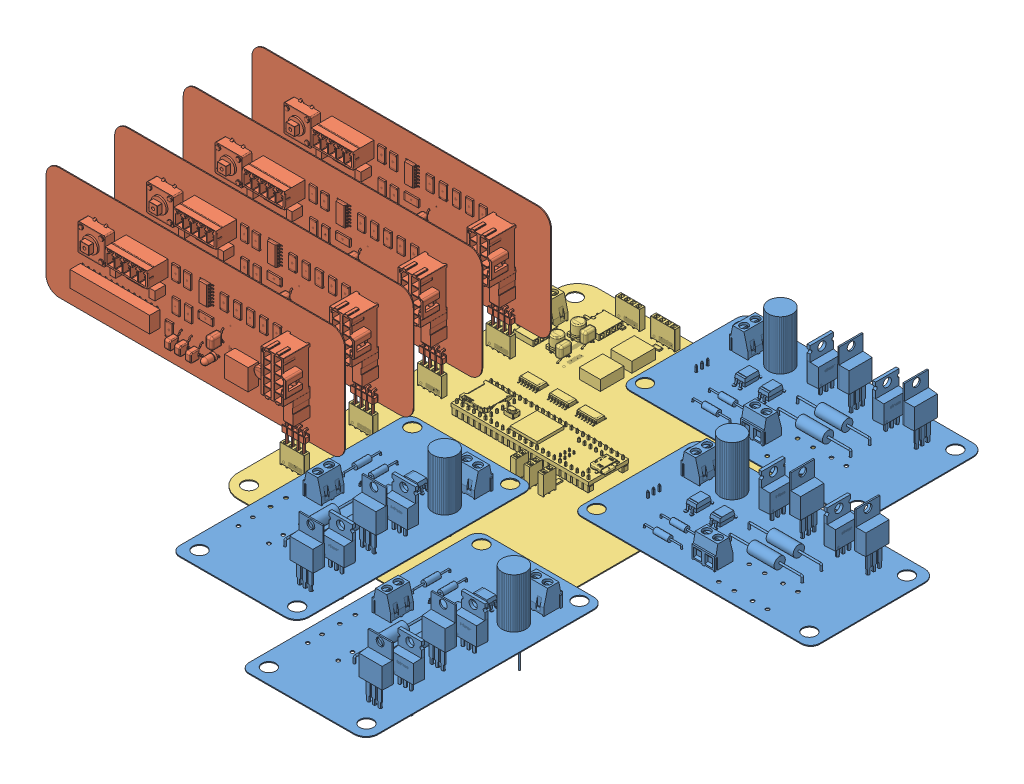
SolidWorks assembly control_sys, configuration Default. Lengths in mm.
Overall size (305.32 69.08 249.07).
9 component instances, 3 part files, 24 mates.
Components (placement in the parent):
- MotorDriver-1: MotorDriver [Default] at (200.9515 -79.5746 394.4399) x (0 0 1) z (0 1 0) size (105.76 55.96 41.98)
- EncoderBoard-2: EncoderBoard [Default] at (182.9184 5.4778 343.1316) x (-1 0 0) z (0 0 1) size (132.47 55.41 21)
- EncoderBoard-3: EncoderBoard [Default] at (182.9184 5.4778 312.694) x (-1 0 0) z (0 0 1) size (132.47 55.41 21)
- EncoderBoard-4: EncoderBoard [Default] at (182.9184 5.4778 373.5693) x (-1 0 0) z (0 0 1) size (132.47 55.41 21)
- EncoderBoard-5: EncoderBoard [Default] at (182.9184 5.4778 404.007) x (-1 0 0) z (0 0 1) size (132.47 55.41 21)
- MotorDriver-2: MotorDriver [Default] at (214.3933 -79.5746 374.1399) x (1 0 0) z (0 1 0) size (105.76 55.96 41.98)
- MotorDriver-3: MotorDriver [Default] at (140.6265 -79.5746 364.8489) x (0 0 1) z (0 1 0) size (105.76 55.96 41.98)
- MotorDriver-4: MotorDriver [Default] at (176.8013 -79.5746 315.0849) x (1 0 0) z (0 1 0) size (105.76 55.96 41.98)
- MotherBoardPCB (1)-1: MotherBoardPCB (1) [Default] at (93.7634 -90.0521 242.695) x (0 0 1) z (0 1 0) size (160.64 119 16.7)
Mates (geometry in assembly coordinates):
- Coincident6: coincident aligned: plane of MotorDriver-2 through (228.7643 -80.4861 349.2519) normal (-1 0 0); plane of MotherBoardPCB (1)-1 through (228.7643 -82.6861 349.5019) normal (-1 0 0)
- Coincident7: coincident aligned: plane of MotorDriver-2 through (229.2643 -80.4861 341.8819) normal (0 0 -1); plane of MotherBoardPCB (1)-1 through (228.7643 -82.6861 341.8819) normal (0 0 -1)
- Coincident8: coincident anti-aligned: plane of MotorDriver-2 through (230.0143 -82.6861 345.6919) normal (0 -1 0); plane of MotherBoardPCB (1)-1 through (231.3043 -82.6861 349.5019) normal (0 1 0)
- Coincident10: coincident aligned: plane of MotorDriver-1 through (225.8395 -80.4861 408.8109) normal (0 0 -1); plane of MotherBoardPCB (1)-1 through (225.5895 -82.6861 408.8109) normal (0 0 -1)
- Coincident11: coincident aligned: plane of MotorDriver-1 through (233.2095 -80.4861 409.3109) normal (1 0 0); plane of MotherBoardPCB (1)-1 through (233.2095 -82.6861 408.8109) normal (1 0 0)
- Coincident12: coincident anti-aligned: plane of MotorDriver-1 through (229.3995 -82.6861 410.0609) normal (0 -1 0); plane of MotherBoardPCB (1)-1 through (225.5895 -82.6861 411.3509) normal (0 1 0)
- Coincident13: coincident aligned: plane of MotorDriver-3 through (165.5145 -80.4861 379.2199) normal (0 0 -1); plane of MotherBoardPCB (1)-1 through (165.2645 -82.6861 379.2199) normal (0 0 -1)
- Coincident14: coincident aligned: plane of MotorDriver-3 through (172.8845 -80.4861 379.7199) normal (1 0 0); plane of MotherBoardPCB (1)-1 through (172.8845 -82.6861 379.2199) normal (1 0 0)
- Coincident15: coincident anti-aligned: plane of MotorDriver-3 through (169.0745 -82.6861 380.4699) normal (0 -1 0); plane of MotherBoardPCB (1)-1 through (165.2645 -82.6861 381.7599) normal (0 1 0)
- Coincident16: coincident aligned: plane of MotorDriver-4 through (191.1723 -80.4861 290.1969) normal (-1 0 0); plane of MotherBoardPCB (1)-1 through (191.1723 -82.6861 290.4469) normal (-1 0 0)
- Coincident17: coincident aligned: plane of MotorDriver-4 through (191.6723 -80.4861 282.8269) normal (0 0 -1); plane of MotherBoardPCB (1)-1 through (191.1723 -82.6861 282.8269) normal (0 0 -1)
- Coincident18: coincident anti-aligned: plane of MotorDriver-4 through (192.4223 -82.6861 286.6369) normal (0 -1 0); plane of MotherBoardPCB (1)-1 through (193.7123 -82.6861 290.4469) normal (0 1 0)
- Coincident19: coincident aligned: plane of EncoderBoard-5 through (130.8484 -75.8021 406.587) normal (0 0 1); plane of MotherBoardPCB (1)-1 through (129.3234 -85.7321 406.587) normal (0 0 1)
- Coincident20: coincident aligned: plane of EncoderBoard-5 through (135.9284 -74.5321 406.587) normal (1 0 0); plane of MotherBoardPCB (1)-1 through (135.9284 -81.4121 405.382) normal (1 0 0)
- Coincident23: coincident anti-aligned: plane of EncoderBoard-5 through (134.3384 -83.0721 404.997) normal (0 -1 0); plane of MotherBoardPCB (1)-1 through (134.4034 -83.0721 405.382) normal (0 1 0)
- Coincident24: coincident aligned: plane of EncoderBoard-4 through (130.8484 -75.8021 376.1493) normal (0 0 1); plane of MotherBoardPCB (1)-1 through (129.3234 -85.7321 376.1493) normal (0 0 1)
- Coincident25: coincident aligned: plane of EncoderBoard-4 through (135.9284 -74.5321 376.1493) normal (1 0 0); plane of MotherBoardPCB (1)-1 through (135.9284 -81.4121 374.9443) normal (1 0 0)
- Coincident26: coincident anti-aligned: plane of EncoderBoard-4 through (126.7184 -83.0721 374.5593) normal (0 -1 0); plane of MotherBoardPCB (1)-1 through (126.7834 -83.0721 374.9443) normal (0 1 0)
- Coincident27: coincident aligned: plane of EncoderBoard-2 through (130.8484 -75.8021 345.7116) normal (0 0 1); plane of MotherBoardPCB (1)-1 through (129.3234 -85.7321 345.7116) normal (0 0 1)
- Coincident28: coincident aligned: plane of EncoderBoard-2 through (135.9284 -74.5321 345.7116) normal (1 0 0); plane of MotherBoardPCB (1)-1 through (135.9284 -81.4121 344.5066) normal (1 0 0)
- Coincident29: coincident anti-aligned: plane of EncoderBoard-2 through (126.7184 -83.0721 344.1216) normal (0 -1 0); plane of MotherBoardPCB (1)-1 through (126.7834 -83.0721 344.5066) normal (0 1 0)
- Coincident30: coincident aligned: plane of EncoderBoard-3 through (135.9284 -74.5321 315.274) normal (1 0 0); plane of MotherBoardPCB (1)-1 through (135.9284 -81.4121 314.069) normal (1 0 0)
- Coincident32: coincident aligned: plane of EncoderBoard-3 through (130.8484 -75.8021 315.274) normal (0 0 1); plane of MotherBoardPCB (1)-1 through (129.3234 -85.7321 315.274) normal (0 0 1)
- Coincident33: coincident anti-aligned: plane of EncoderBoard-3 through (134.3384 -83.0721 313.684) normal (0 -1 0); plane of MotherBoardPCB (1)-1 through (134.4034 -83.0721 314.069) normal (0 1 0)
